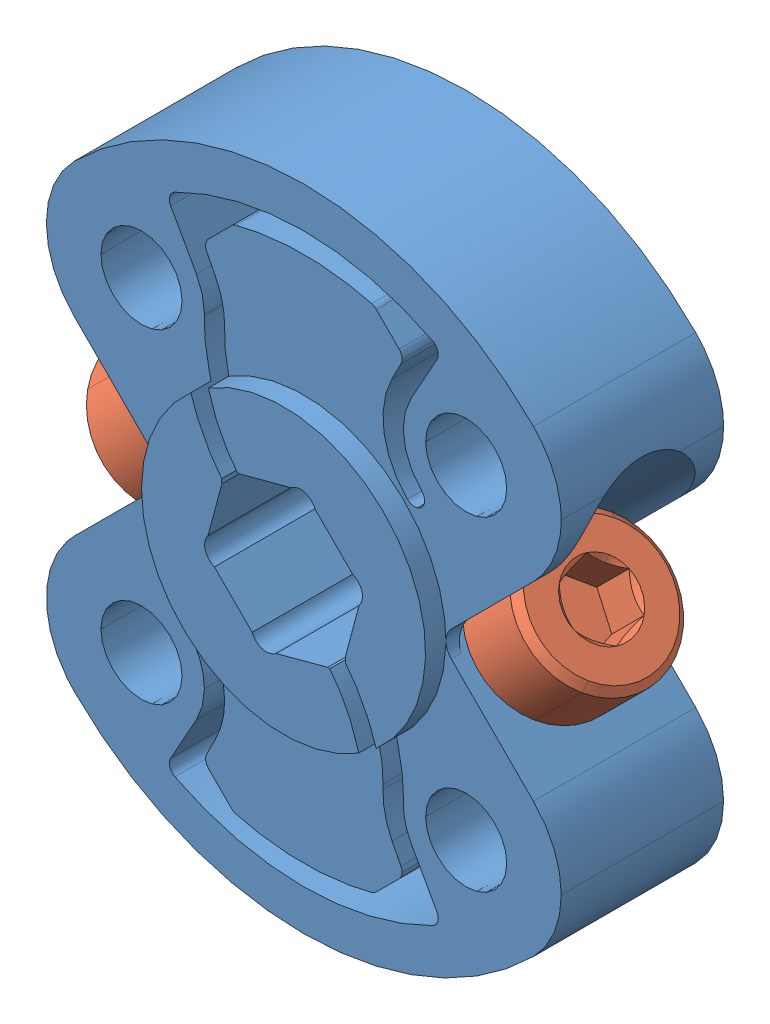
SolidWorks assembly 1311-0016-4008 assembly, configuration Default. Lengths in mm.
Overall size (28.36 32 9.95).
4 component instances, 2 part files, 0 mates.
Components (placement in the parent):
- 1311-0016-4008 assembly.STEP-1: 1311-0016-4008 assembly.STEP [Default] at origin size (28.36 32 9.95)
  - 1311-0016-4008.STEP-1: 1311-0016-4008.STEP [Default] at (-46.6459 19.0262 11.1883) size (25.38 32 9)
  - 2800-0004-0014_90128A207.STEP-1: 2800-0004-0014_90128A207.STEP [Default] at (-48.6988 7.9075 11.1883) x (0.5 -0.5 0.707107) z (-0.707107 -0.707107 0) size (7 7 18.01)
  - 2800-0004-0014_90128A207.STEP-2: 2800-0004-0014_90128A207.STEP [Default] at (-44.5931 30.1449 11.1883) x (-0.5 0.5 0.707107) z (0.707107 0.707107 0) size (7 7 18.01)
